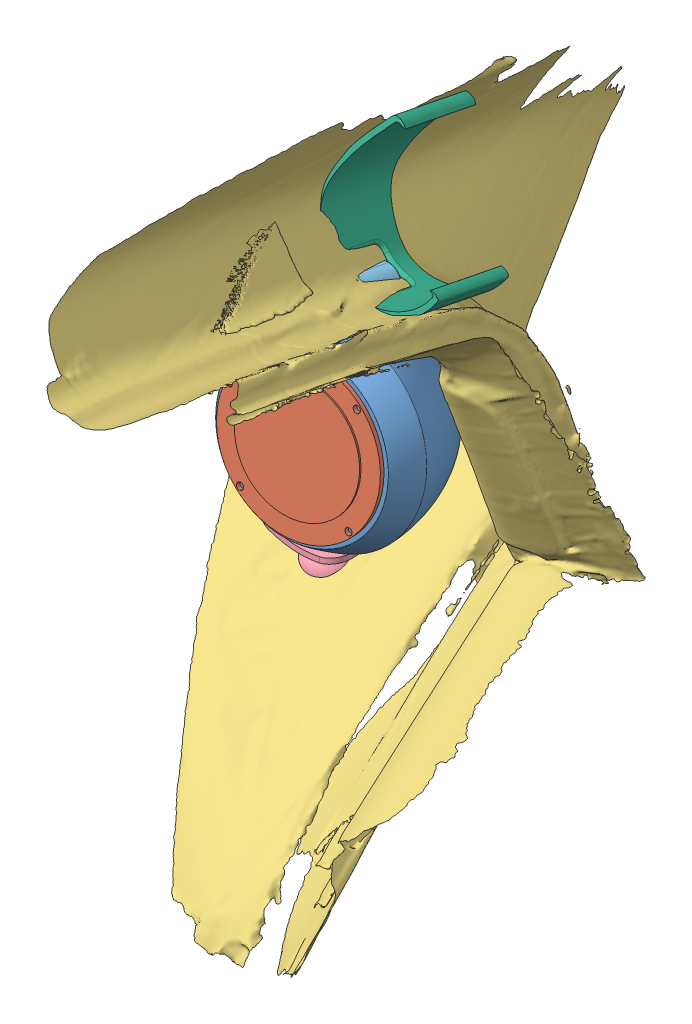
SolidWorks assembly 汽车音箱组装, configuration Default. Lengths in mm.
Overall size (276.78 370.21 467.74).
7 component instances, 7 part files, 7 mates.
Components (placement in the parent):
- 汽车音箱-1: 汽车音箱 [Default] at (-91.8871 103.1436 96.5736) x (-0.16694 -0.972987 0.15946) z (0.979598 -0.182031 -0.08516) size (109.81 81.39 109.81)
- 莞音3寸圆-1: 莞音3寸圆 [Default] at (-91.6074 103.4986 99.0324) x (0.737936 -0.674736 0.013463) z (0.665531 0.724272 -0.180273) size (89 52 89)
- focus_a-1: focus_a [Default] at (-114.0656 67.5174 400.1558) size (276.78 370.21 467.74)
- 音箱支架-1: 音箱支架 [默认] at (-95.4264 99.611 86.8656) x (-0.102085 -0.989529 0.10203) z (0.994015 -0.105479 -0.028427) size (72.81 71.31 73.22)
- 音箱支架-上-1: 音箱支架-上 [默认] at (-95.1032 100.8709 88.063) x (0.094521 0.978979 -0.180735) z (-0.991025 0.109769 0.076292) size (81.67 77.18 111.81)
- focus_a_a_clear-2-1: focus_a_a_clear-2 [默认] at (-130.0431 34.621 300.5846) size (76.52 108.75 76.33)
- 音箱支架-底座-1: 音箱支架-底座 [默认] at (-104.1706 21.0503 66.8571) x (0.999278 0.014493 0.035114) z (-0.026322 -0.402286 0.915136) size (40 25 40)
Mates (geometry in assembly coordinates):
- Concentric1: concentric anti-aligned: cylinder of 汽车音箱-1 through (-92.2227 102.7177 93.623) axis (0.111886 0.14199 0.983524) radius 36.5; cone of 莞音3寸圆-1 through (-91.8871 103.1436 96.5736) axis (-0.111886 -0.14199 -0.983524)
- Coincident1: coincident anti-aligned: plane of 汽车音箱-1 through (-91.8871 103.1436 96.5736) normal (0.111886 0.14199 0.983524); plane of 莞音3寸圆-1 through (-91.8871 103.1436 96.5736) normal (-0.111886 -0.14199 -0.983524)
- 同心1: concentric anti-aligned: cylinder of 音箱支架-上-1 through (-96.6528 152.1493 -5.845) axis (0.10389 0.273291 0.956305) radius 1.75; cylinder of focus_a_a_clear-2-1 through (-87.048 177.4155 82.567) axis (-0.10389 -0.273291 -0.956305) radius 1.6
- 重合1: coincident anti-aligned: plane of 音箱支架-上-1 through (-97.574 182.4011 69.7375) normal (0.10389 0.273291 0.956305); plane of focus_a_a_clear-2-1 through (-88.2947 174.136 71.0913) normal (-0.10389 -0.273291 -0.956305)
- 锁定2: lock: unknown of 汽车音箱-1; unknown of 音箱支架-上-1
- 相切1: tangent aligned: torus of 音箱支架-1; sphere of 音箱支架-底座-1
- 锁定3: lock: unknown of 汽车音箱-1; unknown of 音箱支架-1
